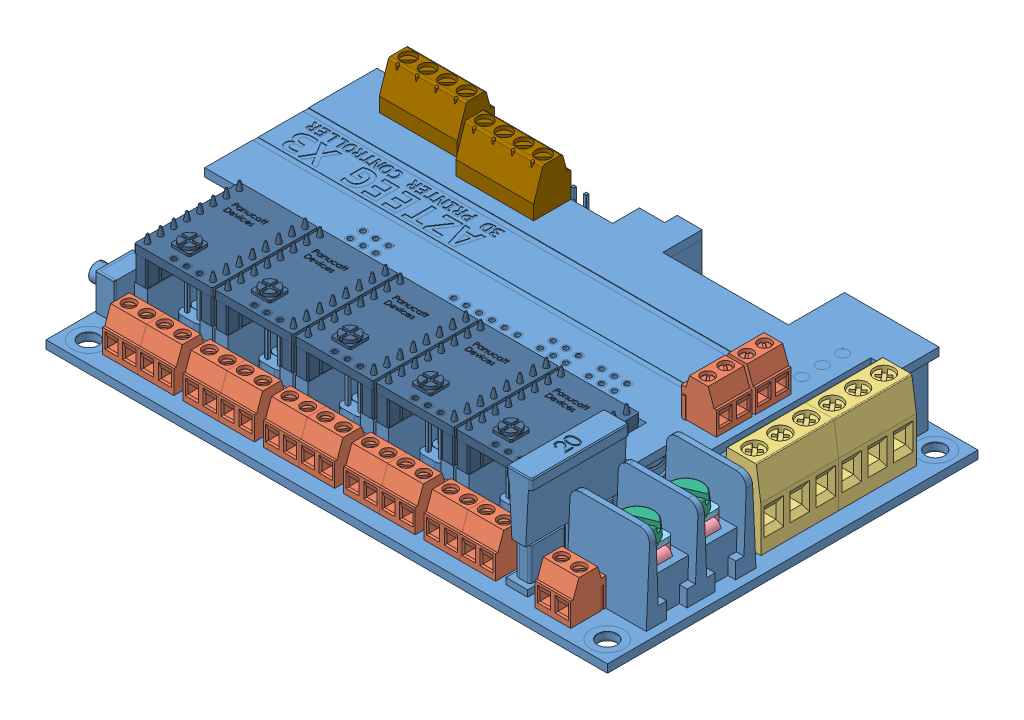
SolidWorks assembly Azteeg X3, configuration Default. Lengths in mm.
Overall size (113.2 25.22 72.75).
37 component instances, 12 part files, 25 mates.
Components (placement in the parent):
- Base_PCB-1: Base_PCB [Default] at (0 0.8 -36.3) x (1 0 0) z (0 1 0) size (113.2 72.75 22.05)
- 2 Way PCB Screw Terminal Block 3_5mm-1: 2 Way PCB Screw Terminal Block 3_5mm [Default] at (-12.81 1.6 -5.55) x (-1 0 0) z (0 1 0) size (7.17 6.89 11.02)
- 3 Way PCB Screw Terminal Block 5_08mm-1: 3 Way PCB Screw Terminal Block 5_08mm [Default] at (-12.25 1.6 -33.3) size (9 15.2 15.24)
- 3 Way PCB Screw Terminal Block 5_08mm-2: 3 Way PCB Screw Terminal Block 5_08mm [Default] at (-12.25 1.6 -48.54) size (9 15.2 15.24)
- SWP (Montage draad)-1: SWP (Montage draad) [Default] at (-9.5 10.15 -15.3077) x (0 0 1) z (0 1 0) size (7 9.9 4.25)
- SWP (Montage draad 2)-1: SWP (Montage draad 2) [Default] at (-9.5 10.15 -15.3077) x (1 0 0) z (0 1 0) size (7 7 1)
- Slotted Cheese Head Screw_DIN_ISO 1207 - M4 x 8 --- 8N-1: Slotted Cheese Head Screw_DIN_ISO 1207 - M4 x 8 --- 8N [Default] at (-9.5 13.75 -15.3077) x (0 -1 0) z (0.926758 0 -0.375659) size (10.61 7 7)
- SWP (Montage draad)-2: SWP (Montage draad) [Default] at (-9.5 10.15 -24.8077) x (0 0 1) z (0 1 0) size (7 9.9 4.25)
- SWP (Montage draad 2)-2: SWP (Montage draad 2) [Default] at (-9.5 10.15 -24.8077) x (1 0 0) z (0 1 0) size (7 7 1)
- Slotted Cheese Head Screw_DIN_ISO 1207 - M4 x 8 --- 8N-2: Slotted Cheese Head Screw_DIN_ISO 1207 - M4 x 8 --- 8N [Default] at (-9.5 13.75 -24.8077) x (0 -1 0) z (0.926758 0 -0.375659) size (10.61 7 7)
- Micro SD Slot___ _________-1: Micro SD Slot___ _________ [Default] at (-101 1.6 -41) x (0 0 1) z (-1 0 0) size (14.25 1.9 15.2)
- USB-Mini-B-1: USB-Mini-B [Default] at (-110 3.6 -53.25) x (0 0 1) z (-1 0 0) size (7.7 3.96 9)
- 2 Way PCB Screw Terminal Block 3_5mm-2: 2 Way PCB Screw Terminal Block 3_5mm [Default] at (-17.4 15.1 -38.82) x (0 0 1) z (0 1 0) size (7.17 6.89 11.02)
- 2 Way PCB Screw Terminal Block 3_5mm-3: 2 Way PCB Screw Terminal Block 3_5mm [Default] at (-17.4 15.1 -46.44) x (0 0 1) z (0 1 0) size (7.17 6.89 11.02)
- 4 Way PCB Screw Terminal Block 3_81mm_Défaut-1: 4 Way PCB Screw Terminal Block 3_81mm_Défaut [Default] at (-87.15 15.1 -65) x (0 0 -1) z (1 0 0) size (7.3 8.5 15.24)
- 4 Way PCB Screw Terminal Block 3_81mm_Défaut-2: 4 Way PCB Screw Terminal Block 3_81mm_Défaut [Default] at (-68.91 15.1 -61.75) x (0 0 -1) z (1 0 0) size (7.3 8.5 15.24)
- Stepper_Driver-1: Stepper_Driver [Default] at (-95 16.7 -30.635) x (1 0 0) z (0 1 0) size (15.25 20.7 14.1)
- Stepper_Driver-2: Stepper_Driver [Default] at (-79.25 16.7 -30.635) x (1 0 0) z (0 1 0) size (15.25 20.7 14.1)
- Stepper_Driver-3: Stepper_Driver [Default] at (-63.5 16.7 -30.635) x (1 0 0) z (0 1 0) size (15.25 20.7 14.1)
- Stepper_Driver-4: Stepper_Driver [Default] at (-47.75 16.7 -30.635) x (1 0 0) z (0 1 0) size (15.25 20.7 14.1)
- Stepper_Driver-5: Stepper_Driver [Default] at (-32 16.7 -30.635) x (1 0 0) z (0 1 0) size (15.25 20.7 14.1)
- 2 Way PCB Screw Terminal Block 3_5mm-4: 2 Way PCB Screw Terminal Block 3_5mm [Default] at (-28.5 1.2818 -6.5036) x (-1 0 0) z (0 1 0) size (7.17 6.89 11.02)
- 2 Way PCB Screw Terminal Block 3_5mm-22: 2 Way PCB Screw Terminal Block 3_5mm [Default] at (-35.5 1.2818 -6.5036) x (-1 0 0) z (0 1 0) size (7.17 6.89 11.02)
- 2 Way PCB Screw Terminal Block 3_5mm-23: 2 Way PCB Screw Terminal Block 3_5mm [Default] at (-51.25 1.2818 -6.5036) x (-1 0 0) z (0 1 0) size (7.17 6.89 11.02)
- 2 Way PCB Screw Terminal Block 3_5mm-24: 2 Way PCB Screw Terminal Block 3_5mm [Default] at (-67 1.2818 -6.5036) x (-1 0 0) z (0 1 0) size (7.17 6.89 11.02)
- 2 Way PCB Screw Terminal Block 3_5mm-25: 2 Way PCB Screw Terminal Block 3_5mm [Default] at (-82.75 1.2818 -6.5036) x (-1 0 0) z (0 1 0) size (7.17 6.89 11.02)
- 2 Way PCB Screw Terminal Block 3_5mm-26: 2 Way PCB Screw Terminal Block 3_5mm [Default] at (-98.5 1.2818 -6.5036) x (-1 0 0) z (0 1 0) size (7.17 6.89 11.02)
- 2 Way PCB Screw Terminal Block 3_5mm-18: 2 Way PCB Screw Terminal Block 3_5mm [Default] at (-44.25 1.2818 -6.5036) x (-1 0 0) z (0 1 0) size (7.17 6.89 11.02)
- 2 Way PCB Screw Terminal Block 3_5mm-19: 2 Way PCB Screw Terminal Block 3_5mm [Default] at (-60 1.2818 -6.5036) x (-1 0 0) z (0 1 0) size (7.17 6.89 11.02)
- 2 Way PCB Screw Terminal Block 3_5mm-20: 2 Way PCB Screw Terminal Block 3_5mm [Default] at (-75.75 1.2818 -6.5036) x (-1 0 0) z (0 1 0) size (7.17 6.89 11.02)
- 2 Way PCB Screw Terminal Block 3_5mm-21: 2 Way PCB Screw Terminal Block 3_5mm [Default] at (-91.5 1.2818 -6.5036) x (-1 0 0) z (0 1 0) size (7.17 6.89 11.02)
- 3 Way PCB Screw Terminal Block 2.5mm_Défaut-1: 3 Way PCB Screw Terminal Block 2.5mm_Défaut [Default] at (-20.4768 0.3168 -71.7207) x (0 0 -1) z (1 0 0) size (4.79 5.58 7.5)
- 3 Way PCB Screw Terminal Block 2.5mm_Défaut-2: 3 Way PCB Screw Terminal Block 2.5mm_Défaut [Default] at (-28.7268 0.3168 -71.7207) x (0 0 -1) z (1 0 0) size (4.79 5.58 7.5)
- 3 Way PCB Screw Terminal Block 2.5mm_Défaut-3: 3 Way PCB Screw Terminal Block 2.5mm_Défaut [Default] at (-36.9768 0.3168 -71.7207) x (0 0 -1) z (1 0 0) size (4.79 5.58 7.5)
- 2 Way PCB Screw Terminal Block 2.5mm_Défaut-1: 2 Way PCB Screw Terminal Block 2.5mm_Défaut [Default] at (-76.3218 0.3165 -71.7205) x (0 0 -1) z (1 0 0) size (4.79 5.58 5)
- 2 Way PCB Screw Terminal Block 2.5mm_Défaut-2: 2 Way PCB Screw Terminal Block 2.5mm_Défaut [Default] at (-81.5718 0.3165 -71.7205) x (0 0 -1) z (1 0 0) size (4.79 5.58 5)
- 2 Way PCB Screw Terminal Block 2.5mm_Défaut-3: 2 Way PCB Screw Terminal Block 2.5mm_Défaut [Default] at (-86.8218 0.3165 -71.7205) x (0 0 -1) z (1 0 0) size (4.79 5.58 5)
Mates (geometry in assembly coordinates):
- Coincident2: coincident anti-aligned: plane of Base_PCB-1 through (0 1.6 -36.3) normal (0 1 0); plane of 2 Way PCB Screw Terminal Block 3_5mm-4 through (-32.0009 1.6 -9.9615) normal (0 -1 0)
- Parallel1: parallel aligned: plane of Base_PCB-1 through (-110 1.6 0) normal (0 0 1); plane of 2 Way PCB Screw Terminal Block 3_5mm-4 through (-32.0009 1.6 -3.0717) normal (0 0 1)
- Coincident5: coincident aligned: plane of 2 Way PCB Screw Terminal Block 3_5mm-4 through (-32.0009 1.6 -3.0717) normal (0 0 1); plane of 2 Way PCB Screw Terminal Block 3_5mm-22 through (-39.0009 1.6 -3.0717) normal (0 0 1)
- Coincident6: coincident anti-aligned: plane of Base_PCB-1 through (0 1.6 -36.3) normal (0 1 0); plane of 2 Way PCB Screw Terminal Block 3_5mm-22 through (-39.0009 1.6 -9.9615) normal (0 -1 0)
- Coincident9: coincident: line of Base_PCB-1 through (-30.25 0 -6.5) axis (1 0 0); plane of 2 Way PCB Screw Terminal Block 3_5mm-4 through (-28.5 1.2818 -6.5) normal (0 0 -1)
- Coincident10: coincident: point of Base_PCB-1; plane of 2 Way PCB Screw Terminal Block 3_5mm-4
- Coincident11: coincident: point of Base_PCB-1; plane of 2 Way PCB Screw Terminal Block 3_5mm-22
- Coincident12: coincident anti-aligned: plane of Base_PCB-1 through (0 1.6 -36.3) normal (0 1 0); plane of 3 Way PCB Screw Terminal Block 2.5mm_Défaut-1 through (-27.7034 1.6 -65.6394) normal (0 -1 0)
- Coincident13: coincident anti-aligned: plane of Base_PCB-1 through (0 1.6 -36.3) normal (0 1 0); plane of 3 Way PCB Screw Terminal Block 2.5mm_Défaut-2 through (-35.9534 1.6 -65.6394) normal (0 -1 0)
- Coincident14: coincident anti-aligned: plane of Base_PCB-1 through (0 1.6 -36.3) normal (0 1 0); plane of 3 Way PCB Screw Terminal Block 2.5mm_Défaut-3 through (-44.2034 1.6 -65.6394) normal (0 -1 0)
- Concentric4: concentric anti-aligned: cylinder of Base_PCB-1 through (-27.5 1.6 -68.1) axis (0 -1 0) radius 0.5; cylinder of 3 Way PCB Screw Terminal Block 2.5mm_Défaut-1 through (-27.5 6.6787 -68.1) axis (0 1 0) radius 0.9514
- Concentric5: concentric anti-aligned: cylinder of Base_PCB-1 through (-32.5 1.6 -68.1) axis (0 -1 0) radius 0.5; cylinder of 3 Way PCB Screw Terminal Block 2.5mm_Défaut-1 through (-32.5 6.6787 -68.1) axis (0 1 0) radius 0.9514
- Concentric6: concentric anti-aligned: cylinder of Base_PCB-1 through (-35.75 1.6 -68.1) axis (0 -1 0) radius 0.5; cylinder of 3 Way PCB Screw Terminal Block 2.5mm_Défaut-2 through (-35.75 6.6787 -68.1) axis (0 1 0) radius 0.9514
- Concentric7: concentric anti-aligned: cylinder of Base_PCB-1 through (-40.75 1.6 -68.1) axis (0 -1 0) radius 0.5; cylinder of 3 Way PCB Screw Terminal Block 2.5mm_Défaut-2 through (-40.75 6.6787 -68.1) axis (0 1 0) radius 0.9514
- Concentric8: concentric anti-aligned: cylinder of Base_PCB-1 through (-44 1.6 -68.1) axis (0 -1 0) radius 0.5; cylinder of 3 Way PCB Screw Terminal Block 2.5mm_Défaut-3 through (-44 6.6787 -68.1) axis (0 1 0) radius 0.9514
- Concentric9: concentric anti-aligned: cylinder of Base_PCB-1 through (-49 1.6 -68.1) axis (0 -1 0) radius 0.5; cylinder of 3 Way PCB Screw Terminal Block 2.5mm_Défaut-3 through (-49 6.6787 -68.1) axis (0 1 0) radius 0.9514
- Coincident15: coincident anti-aligned: plane of Base_PCB-1 through (0 1.6 -36.3) normal (0 1 0); plane of 2 Way PCB Screw Terminal Block 2.5mm_Défaut-1 through (-84.2034 1.6 -65.6394) normal (0 -1 0)
- Coincident16: coincident anti-aligned: plane of Base_PCB-1 through (0 1.6 -36.3) normal (0 1 0); plane of 2 Way PCB Screw Terminal Block 2.5mm_Défaut-2 through (-89.4534 1.6 -65.6394) normal (0 -1 0)
- Coincident17: coincident anti-aligned: plane of Base_PCB-1 through (0 1.6 -36.3) normal (0 1 0); plane of 2 Way PCB Screw Terminal Block 2.5mm_Défaut-3 through (-94.7034 1.6 -65.6394) normal (0 -1 0)
- Concentric10: concentric anti-aligned: cylinder of Base_PCB-1 through (-86.5 1.6 -68.1) axis (0 -1 0) radius 0.5; cylinder of 2 Way PCB Screw Terminal Block 2.5mm_Défaut-1 through (-86.5 6.6787 -68.1) axis (0 1 0) radius 0.9514
- Concentric11: concentric anti-aligned: cylinder of Base_PCB-1 through (-89 1.6 -68.1) axis (0 -1 0) radius 0.5; cylinder of 2 Way PCB Screw Terminal Block 2.5mm_Défaut-1 through (-89 6.6787 -68.1) axis (0 1 0) radius 0.9514
- Concentric12: concentric anti-aligned: cylinder of Base_PCB-1 through (-91.75 1.6 -68.1) axis (0 -1 0) radius 0.5; cylinder of 2 Way PCB Screw Terminal Block 2.5mm_Défaut-2 through (-91.75 6.6787 -68.1) axis (0 1 0) radius 0.9514
- Concentric13: concentric anti-aligned: cylinder of Base_PCB-1 through (-94.25 1.6 -68.1) axis (0 -1 0) radius 0.5; cylinder of 2 Way PCB Screw Terminal Block 2.5mm_Défaut-2 through (-94.25 6.6787 -68.1) axis (0 1 0) radius 0.9514
- Concentric14: concentric anti-aligned: cylinder of Base_PCB-1 through (-97 1.6 -68.1) axis (0 -1 0) radius 0.5; cylinder of 2 Way PCB Screw Terminal Block 2.5mm_Défaut-3 through (-97 6.6787 -68.1) axis (0 1 0) radius 0.9514
- Concentric15: concentric anti-aligned: cylinder of Base_PCB-1 through (-99.5 1.6 -68.1) axis (0 -1 0) radius 0.5; cylinder of 2 Way PCB Screw Terminal Block 2.5mm_Défaut-3 through (-99.5 6.6787 -68.1) axis (0 1 0) radius 0.9514
